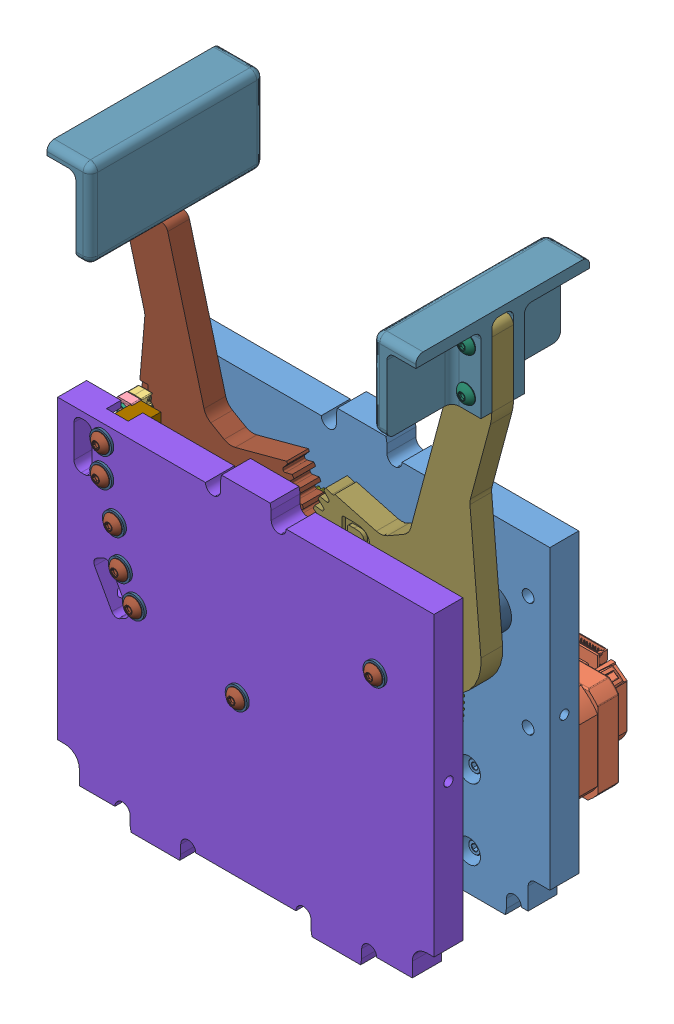
SolidWorks assembly R_ASSY_200_rev3, configuration Default. Lengths in mm.
Overall size (165.1 249.75 130.56).
101 component instances, 30 part files, 189 mates.
Components (placement in the parent):
- R_200_01_rev3-1: R_200_01_rev3 [Default] at (42.4652 115.7578 110.3805) size (165.1 155.57 12.7)
- STP-MTR-17048E-1: STP-MTR-17048E [Default] at (114.3442 119.6359 5.7474) x (-1 0 0) z (0 0 1) size (42.16 62.89 84.58)
- R_200_03_rev2-1: R_200_03_rev2 [Default] at (39.2022 113.0052 142.1305) x (-0.709234 0.704973 0) z (0 0 1) size (6.35 6.35 50.8)
- R_200_04-1: R_200_04 [Default] at (-14.6848 152.2703 142.1305) x (0.39149 -0.920182 0) z (0 0 -1) size (9.53 9.53 50.8)
- R_200_04-2: R_200_04 [Default] at (99.6152 152.2703 142.1305) x (0.332871 0.942972 0) z (0 0 1) size (9.53 9.53 50.8)
- 91116A120_TYPE 18-8 STAINLESS STL OVERSIZED FLAT WASHER-1: 91116A120_TYPE 18-8 STAINLESS STL OVERSIZED FLAT WASHER [91116A120] at (-20.6538 89.9768 116.7305) size (9 9 0.9)
- 91116A120_TYPE 18-8 STAINLESS STL OVERSIZED FLAT WASHER-9: 91116A120_TYPE 18-8 STAINLESS STL OVERSIZED FLAT WASHER [91116A120] at (105.5842 89.9768 116.7305) x (0.949722 0.313094 0) z (0 0 1) size (9 9 0.9)
- 91116A120_TYPE 18-8 STAINLESS STL OVERSIZED FLAT WASHER-11: 91116A120_TYPE 18-8 STAINLESS STL OVERSIZED FLAT WASHER [91116A120] at (105.5842 58.9888 116.7305) x (0.902124 0.431476 0) z (0 0 1) size (9 9 0.9)
- 12t_Steel_Spur_Gear_32_DP_RS775_Motor_217-5859.step-1: 12t_Steel_Spur_Gear_32_DP_RS775_Motor_217-5859.step [Default] at (4.3652 69.7203 125.1283) size (10.98 10.98 19.05)
- 12t_Steel_Spur_Gear_32_DP_RS775_Motor_217-5859.step-2: 12t_Steel_Spur_Gear_32_DP_RS775_Motor_217-5859.step [Default] at (74.0391 69.7203 125.1283) size (10.98 10.98 19.05)
- R_200_05-1: R_200_05 [Default] at (39.2022 113.0052 132.6055) x (-0.958932 0.283637 0) z (0 0 -1) size (103.19 103.19 25.4)
- R_200_02_rev3-1: R_200_02_rev3 [Default] at (42.4652 115.7578 161.1805) size (165.1 155.57 12.7)
- R_200_07_SPCR_rev3-1: R_200_07_SPCR_rev3 [Default] at (39.2022 113.0052 153.243) size (12.7 12.7 7.68)
- R_200_09_SPCR_rev3-3: R_200_09_SPCR_rev3 [Default] at (-14.6848 152.2703 135.7805) x (1 0 0) z (0 0 -1) size (17.46 17.46 12.57)
- R_203_01_rev4-1: R_203_01_rev4 [Default] at (-14.6848 152.2703 142.1305) size (82.51 177.51 9.53)
- R_200_09_SPCR_rev3-4: R_200_09_SPCR_rev3 [Default] at (99.6152 152.2703 123.2075) x (0.999677 -0.025413 0) z (0 0 1) size (17.46 17.46 12.57)
- R_203_02_rev4-1: R_203_02_rev4 [Default] at (99.6152 152.2703 142.1305) x (-1 0 0) z (0 0 -1) size (82.48 176.02 9.53)
- STP-MTR-17048E-2: STP-MTR-17048E [Default] at (44.6703 119.6359 5.7474) x (-1 0 0) z (0 0 1) size (42.16 62.89 84.58)
- 91125A453_18-8 SS FEM THRDED ROUND STANDOFF-1: 91125A453_18-8 SS FEM THRDED ROUND STANDOFF [91125A453] at (-32.103 275.0161 142.1305) x (-1 0 0) z (0 0 1) size (6.35 6.35 10.62)
- 91125A453_18-8 SS FEM THRDED ROUND STANDOFF-2: 91125A453_18-8 SS FEM THRDED ROUND STANDOFF [91125A453] at (-32.103 255.9661 142.1305) x (-0.987351 -0.158553 0) z (0 0 1) size (6.35 6.35 10.62)
- 91125A453_18-8 SS FEM THRDED ROUND STANDOFF-4: 91125A453_18-8 SS FEM THRDED ROUND STANDOFF [91125A453] at (117.0334 275.0161 142.1305) x (-0.34202 0.939693 0) z (0 0 -1) size (6.35 6.35 10.62)
- 91125A453_18-8 SS FEM THRDED ROUND STANDOFF-6: 91125A453_18-8 SS FEM THRDED ROUND STANDOFF [91125A453] at (117.0334 255.9661 142.1305) x (-0.5 0.866025 0) z (0 0 -1) size (6.35 6.35 10.62)
- R_203_05-1: R_203_05 [Default] at (-28.928 268.6661 142.1305) x (0 0 -1) z (1 0 0) size (76.2 38.1 19.05)
- 92949A192_18-8 SS BUTTON HEAD HEX DRIVE SCREW-19: 92949A192_18-8 SS BUTTON HEAD HEX DRIVE SCREW [92949A192] at (-32.103 275.0161 147.9979) x (-0.998312 -0.058087 0) z (0 0 1) size (7.92 7.92 12.15)
- 92949A192_18-8 SS BUTTON HEAD HEX DRIVE SCREW-20: 92949A192_18-8 SS BUTTON HEAD HEX DRIVE SCREW [92949A192] at (-32.103 255.9661 147.9979) x (-0.976474 -0.215637 0) z (0 0 1) size (7.92 7.92 12.15)
- 92949A192_18-8 SS BUTTON HEAD HEX DRIVE SCREW-22: 92949A192_18-8 SS BUTTON HEAD HEX DRIVE SCREW [92949A192] at (-32.103 275.0161 136.2631) x (0.973943 -0.226793 0) z (0 0 -1) size (7.92 7.92 12.15)
- 92949A192_18-8 SS BUTTON HEAD HEX DRIVE SCREW-25: 92949A192_18-8 SS BUTTON HEAD HEX DRIVE SCREW [92949A192] at (-32.103 255.9661 136.2631) x (0.948563 -0.316589 0) z (0 0 -1) size (7.92 7.92 12.15)
- 92949A192_18-8 SS BUTTON HEAD HEX DRIVE SCREW-27: 92949A192_18-8 SS BUTTON HEAD HEX DRIVE SCREW [92949A192] at (117.0334 275.0161 147.9979) x (-0.973943 -0.226793 0) z (0 0 1) size (7.92 7.92 12.15)
- 92949A192_18-8 SS BUTTON HEAD HEX DRIVE SCREW-28: 92949A192_18-8 SS BUTTON HEAD HEX DRIVE SCREW [92949A192] at (117.0334 255.9661 147.9979) x (-0.948563 -0.316589 0) z (0 0 1) size (7.92 7.92 12.15)
- 92949A192_18-8 SS BUTTON HEAD HEX DRIVE SCREW-29: 92949A192_18-8 SS BUTTON HEAD HEX DRIVE SCREW [92949A192] at (117.0334 275.0161 136.2631) x (-0.998312 0.058087 0) z (0 0 -1) size (7.92 7.92 12.15)
- 92949A192_18-8 SS BUTTON HEAD HEX DRIVE SCREW-30: 92949A192_18-8 SS BUTTON HEAD HEX DRIVE SCREW [92949A192] at (117.0334 255.9661 136.2631) x (-0.976474 0.215637 0) z (0 0 -1) size (7.92 7.92 12.15)
- R_203_05-2: R_203_05 [Default] at (113.8584 268.6661 142.1305) x (0 0 1) z (-1 0 0) size (76.2 38.1 19.05)
- 2797T100_LIGHT DUTY DRY-RUNNING THRUST BEARING-1: 2797T100_LIGHT DUTY DRY-RUNNING THRUST BEARING [2797T1] at (39.2022 113.0052 123.8742) x (-0.703019 0.711171 0) z (0 0 1) size (15.88 15.88 1.59)
- 6338K413_OIL-EMBEDDED FLANGED SLEEVE BEARING-1: 6338K413_OIL-EMBEDDED FLANGED SLEEVE BEARING [6338K413] at (39.2022 113.0052 124.668) x (1 0 0) z (0 -1 0) size (12.7 12.7 12.7)
- 6338K413_OIL-EMBEDDED FLANGED SLEEVE BEARING-2: 6338K413_OIL-EMBEDDED FLANGED SLEEVE BEARING [6338K413] at (39.2022 113.0052 153.243) x (0.987351 -0.158553 0) z (0.158553 0.987351 0) size (12.7 12.7 12.7)
- 6338K414_OIL-EMBEDDED FLANGED SLEEVE BEARING-1: 6338K414_OIL-EMBEDDED FLANGED SLEEVE BEARING [6338K414] at (-14.6848 152.2703 135.7805) x (0.998098 0.061654 0) z (0.061654 -0.998098 0) size (17.46 6.35 17.46)
- 6338K414_OIL-EMBEDDED FLANGED SLEEVE BEARING-2: 6338K414_OIL-EMBEDDED FLANGED SLEEVE BEARING [6338K414] at (-14.6848 152.2703 148.4805) x (0.995248 -0.097377 0) z (0.097377 0.995248 0) size (17.46 6.35 17.46)
- 6338K414_OIL-EMBEDDED FLANGED SLEEVE BEARING-4: 6338K414_OIL-EMBEDDED FLANGED SLEEVE BEARING [6338K414] at (99.6152 152.2703 148.4805) x (-0.283434 0.958992 0) z (-0.958992 -0.283434 0) size (17.46 6.35 17.46)
- 6338K414_OIL-EMBEDDED FLANGED SLEEVE BEARING-6: 6338K414_OIL-EMBEDDED FLANGED SLEEVE BEARING [6338K414] at (99.6152 152.2703 135.7805) x (-0.552443 -0.833551 0) z (-0.833551 0.552443 0) size (17.46 6.35 17.46)
- R_200_09_SPCR_rev3-5: R_200_09_SPCR_rev3 [Default] at (99.6152 152.2703 161.0535) x (0.966573 0.25639 0) z (0 0 -1) size (17.46 17.46 12.57)
- R_200_09_SPCR_rev3-7: R_200_09_SPCR_rev3 [Default] at (-14.6848 152.2703 161.0535) x (-0.36579 0.930697 0) z (0 0 -1) size (17.46 17.46 12.57)
- 91116A120_TYPE 18-8 STAINLESS STL OVERSIZED FLAT WASHER-12: 91116A120_TYPE 18-8 STAINLESS STL OVERSIZED FLAT WASHER [91116A120] at (89.5331 85.2143 116.7305) size (9 9 0.9)
- 91292A027_TYPE 18-8 SS SOCKET HEAD CAP SCREW-1: 91292A027_TYPE 18-8 SS SOCKET HEAD CAP SCREW [91292A027] at (89.5331 85.2143 103.6305) x (-0.923728 -0.383049 0) z (0 0 -1) size (5.5 5.5 17.24)
- 91292A027_TYPE 18-8 SS SOCKET HEAD CAP SCREW-8: 91292A027_TYPE 18-8 SS SOCKET HEAD CAP SCREW [91292A027] at (89.5331 54.2263 103.6305) x (-0.923728 -0.383049 0) z (0 0 -1) size (5.5 5.5 17.24)
- 91292A027_TYPE 18-8 SS SOCKET HEAD CAP SCREW-9: 91292A027_TYPE 18-8 SS SOCKET HEAD CAP SCREW [91292A027] at (-11.1288 85.2143 103.6305) x (-0.923728 -0.383049 0) z (0 0 -1) size (5.5 5.5 17.24)
- 91292A027_TYPE 18-8 SS SOCKET HEAD CAP SCREW-10: 91292A027_TYPE 18-8 SS SOCKET HEAD CAP SCREW [91292A027] at (58.5451 85.2143 103.6305) x (-0.923728 -0.383049 0) z (0 0 -1) size (5.5 5.5 17.24)
- 91292A027_TYPE 18-8 SS SOCKET HEAD CAP SCREW-11: 91292A027_TYPE 18-8 SS SOCKET HEAD CAP SCREW [91292A027] at (58.5451 54.2263 103.6305) x (-0.923728 -0.383049 0) z (0 0 -1) size (5.5 5.5 17.24)
- 91292A027_TYPE 18-8 SS SOCKET HEAD CAP SCREW-12: 91292A027_TYPE 18-8 SS SOCKET HEAD CAP SCREW [91292A027] at (-11.1288 54.2263 103.6305) x (-0.923728 -0.383049 0) z (0 0 -1) size (5.5 5.5 17.24)
- 91292A027_TYPE 18-8 SS SOCKET HEAD CAP SCREW-13: 91292A027_TYPE 18-8 SS SOCKET HEAD CAP SCREW [91292A027] at (19.8592 54.2263 103.6305) x (-0.923728 -0.383049 0) z (0 0 -1) size (5.5 5.5 17.24)
- 91292A027_TYPE 18-8 SS SOCKET HEAD CAP SCREW-14: 91292A027_TYPE 18-8 SS SOCKET HEAD CAP SCREW [91292A027] at (19.8592 85.2143 103.6305) x (-0.923728 -0.383049 0) z (0 0 -1) size (5.5 5.5 17.24)
- 91116A120_TYPE 18-8 STAINLESS STL OVERSIZED FLAT WASHER-19: 91116A120_TYPE 18-8 STAINLESS STL OVERSIZED FLAT WASHER [91116A120] at (89.5331 54.2263 116.7305) size (9 9 0.9)
- 91116A120_TYPE 18-8 STAINLESS STL OVERSIZED FLAT WASHER-20: 91116A120_TYPE 18-8 STAINLESS STL OVERSIZED FLAT WASHER [91116A120] at (-11.1288 85.2143 116.7305) size (9 9 0.9)
- 91116A120_TYPE 18-8 STAINLESS STL OVERSIZED FLAT WASHER-21: 91116A120_TYPE 18-8 STAINLESS STL OVERSIZED FLAT WASHER [91116A120] at (58.5451 85.2143 116.7305) size (9 9 0.9)
- 91116A120_TYPE 18-8 STAINLESS STL OVERSIZED FLAT WASHER-22: 91116A120_TYPE 18-8 STAINLESS STL OVERSIZED FLAT WASHER [91116A120] at (58.5451 54.2263 116.7305) size (9 9 0.9)
- 91116A120_TYPE 18-8 STAINLESS STL OVERSIZED FLAT WASHER-23: 91116A120_TYPE 18-8 STAINLESS STL OVERSIZED FLAT WASHER [91116A120] at (-11.1288 54.2263 116.7305) size (9 9 0.9)
- 91116A120_TYPE 18-8 STAINLESS STL OVERSIZED FLAT WASHER-24: 91116A120_TYPE 18-8 STAINLESS STL OVERSIZED FLAT WASHER [91116A120] at (19.8592 54.2263 116.7305) size (9 9 0.9)
- 91116A120_TYPE 18-8 STAINLESS STL OVERSIZED FLAT WASHER-25: 91116A120_TYPE 18-8 STAINLESS STL OVERSIZED FLAT WASHER [91116A120] at (19.8592 85.2143 116.7305) size (9 9 0.9)
- dc1c-a1aa-1: dc1c-a1aa [Default] at (-27.4348 169.2553 154.8305) x (0 1 0) z (-1 0 0) size (19.85 14.96 6.45)
  - dc1c-a1aa_01-1: dc1c-a1aa_01 [Default] at origin size (5.58 3.61 5.58)
  - dc1c-a1aa_02-1: dc1c-a1aa_02 [Default] at origin size (19.73 5.96 6.26)
  - dc1c-a1aa_03-1: dc1c-a1aa_03 [Default] at origin size (19.85 3.9 6.45)
  - dc1c-a1aa_04-1: dc1c-a1aa_04 [Default] at origin size (1.69 3.85 2.68)
  - dc1c-a1aa_05-1: dc1c-a1aa_05 [Default] at origin size (1.69 3.85 2.68)
  - dc1c-a1aa_06-1: dc1c-a1aa_06 [Default] at origin size (1.69 3.85 2.68)
- 92095A104_BUTTON HEAD HEX DRIVE SCREW-1: 92095A104_BUTTON HEAD HEX DRIVE SCREW [92095A104] at (-31.5598 169.2553 154.8305) x (0 0 1) z (-1 0 0) size (3.8 3.8 11.02)
- R_200_10-2: R_200_10 [Default] at (-20.241 174.0203 167.5305) x (0 0 1) z (-1 0 0) size (14.29 19.05 9.53)
- 92095A104_BUTTON HEAD HEX DRIVE SCREW-2: 92095A104_BUTTON HEAD HEX DRIVE SCREW [92095A104] at (-31.5598 178.7853 154.8305) x (0 -0.984808 -0.173648) z (-1 0 0) size (3.8 3.8 11.02)
- R_200_10-3: R_200_10 [Default] at (-8.9998 130.5536 167.5305) x (0 0 1) z (-0.87462 -0.48481 0) size (14.29 19.05 9.53)
- dc1c-a1aa-2: dc1c-a1aa [Default] at (-17.6017 131.2336 154.8305) x (0.48481 -0.87462 0) z (0.87462 0.48481 0) size (19.85 14.96 6.45)
  - dc1c-a1aa_01-1: dc1c-a1aa_01 [Default] at origin size (5.58 3.61 5.58)
  - dc1c-a1aa_02-1: dc1c-a1aa_02 [Default] at origin size (19.73 5.96 6.26)
  - dc1c-a1aa_03-1: dc1c-a1aa_03 [Default] at origin size (19.85 3.9 6.45)
  - dc1c-a1aa_04-1: dc1c-a1aa_04 [Default] at origin size (1.69 3.85 2.68)
  - dc1c-a1aa_05-1: dc1c-a1aa_05 [Default] at origin size (1.69 3.85 2.68)
  - dc1c-a1aa_06-1: dc1c-a1aa_06 [Default] at origin size (1.69 3.85 2.68)
- 92095A104_BUTTON HEAD HEX DRIVE SCREW-3: 92095A104_BUTTON HEAD HEX DRIVE SCREW [92095A104] at (-21.2095 129.2337 154.8305) x (-0.34402 0.620628 0.704607) z (-0.87462 -0.48481 0) size (3.8 3.8 11.02)
- 92095A104_BUTTON HEAD HEX DRIVE SCREW-5: 92095A104_BUTTON HEAD HEX DRIVE SCREW [92095A104] at (-16.5893 120.8986 154.8305) x (-0.449843 0.811539 -0.372887) z (-0.87462 -0.48481 0) size (3.8 3.8 11.02)
- 92141A009_TYPE 18-8 STAINLESS STEEL FLAT WASHER-5: 92141A009_TYPE 18-8 STAINLESS STEEL FLAT WASHER [92141A009] at (-20.241 180.3703 174.8965) x (-0.777574 -0.628792 0) z (0.628792 -0.777574 0) size (9.53 1.02 9.53)
- 92949A194_18-8 SS BUTTON HEAD HEX DRIVE SCREW-12: 92949A194_18-8 SS BUTTON HEAD HEX DRIVE SCREW [92949A194] at (-20.241 180.3703 169.6514) x (0.994367 -0.105992 0) z (0 0 1) size (7.92 7.92 15.34)
- 92141A009_TYPE 18-8 STAINLESS STEEL FLAT WASHER-6: 92141A009_TYPE 18-8 STAINLESS STEEL FLAT WASHER [92141A009] at (-20.241 167.6703 174.8965) x (-0.668041 -0.744124 0) z (0.744124 -0.668041 0) size (9.53 1.02 9.53)
- 92949A194_18-8 SS BUTTON HEAD HEX DRIVE SCREW-17: 92949A194_18-8 SS BUTTON HEAD HEX DRIVE SCREW [92949A194] at (-20.241 167.6703 169.6514) x (0.964983 -0.262311 0) z (0 0 1) size (7.92 7.92 15.34)
- 92141A009_TYPE 18-8 STAINLESS STEEL FLAT WASHER-7: 92141A009_TYPE 18-8 STAINLESS STEEL FLAT WASHER [92141A009] at (-14.6848 152.2703 174.8965) x (-0.567853 -0.82313 0) z (0.82313 -0.567853 0) size (9.53 1.02 9.53)
- 92949A194_18-8 SS BUTTON HEAD HEX DRIVE SCREW-18: 92949A194_18-8 SS BUTTON HEAD HEX DRIVE SCREW [92949A194] at (-14.6848 152.2703 169.6514) x (0.923728 -0.383049 0) z (0 0 1) size (7.92 7.92 15.34)
- 92141A009_TYPE 18-8 STAINLESS STEEL FLAT WASHER-8: 92141A009_TYPE 18-8 STAINLESS STEEL FLAT WASHER [92141A009] at (-12.0783 136.1074 174.8965) x (-0.488654 -0.872477 0) z (0.872477 -0.488654 0) size (9.53 1.02 9.53)
- 92949A194_18-8 SS BUTTON HEAD HEX DRIVE SCREW-19: 92949A194_18-8 SS BUTTON HEAD HEX DRIVE SCREW [92949A194] at (-12.0783 136.1074 169.6514) x (0.884001 -0.467484 0) z (0 0 1) size (7.92 7.92 15.34)
- 92141A009_TYPE 18-8 STAINLESS STEEL FLAT WASHER-9: 92141A009_TYPE 18-8 STAINLESS STEEL FLAT WASHER [92141A009] at (-5.9212 124.9998 174.8965) x (-0.440433 -0.897785 0) z (0.897785 -0.440433 0) size (9.53 1.02 9.53)
- 92949A194_18-8 SS BUTTON HEAD HEX DRIVE SCREW-20: 92949A194_18-8 SS BUTTON HEAD HEX DRIVE SCREW [92949A194] at (-5.9212 124.9998 169.6514) x (0.857241 -0.514915 0) z (0 0 1) size (7.92 7.92 15.34)
- 92141A009_TYPE 18-8 STAINLESS STEEL FLAT WASHER-10: 92141A009_TYPE 18-8 STAINLESS STEEL FLAT WASHER [92141A009] at (39.2022 113.0052 174.8965) x (-0.431679 -0.902027 0) z (0.902027 -0.431679 0) size (9.53 1.02 9.53)
- 92949A194_18-8 SS BUTTON HEAD HEX DRIVE SCREW-16: 92949A194_18-8 SS BUTTON HEAD HEX DRIVE SCREW [92949A194] at (39.2022 113.0052 169.6514) x (0.852192 -0.523229 0) z (0 0 1) size (7.92 7.92 15.34)
- 92141A009_TYPE 18-8 STAINLESS STEEL FLAT WASHER-11: 92141A009_TYPE 18-8 STAINLESS STEEL FLAT WASHER [92141A009] at (99.6152 152.2703 174.8965) x (-0.468067 -0.883693 0) z (0.883693 -0.468067 0) size (9.53 1.02 9.53)
- 92949A194_18-8 SS BUTTON HEAD HEX DRIVE SCREW-11: 92949A194_18-8 SS BUTTON HEAD HEX DRIVE SCREW [92949A194] at (99.6152 152.2703 169.6514) x (0.872799 -0.488079 0) z (0 0 1) size (7.92 7.92 15.34)
- 92141A009_TYPE 18-8 STAINLESS STEEL FLAT WASHER-14: 92141A009_TYPE 18-8 STAINLESS STEEL FLAT WASHER [92141A009] at (-14.6848 152.2703 109.3645) x (-0.484215 -0.874949 0) z (-0.874949 0.484215 0) size (9.53 1.02 9.53)
- 92949A194_18-8 SS BUTTON HEAD HEX DRIVE SCREW-22: 92949A194_18-8 SS BUTTON HEAD HEX DRIVE SCREW [92949A194] at (-14.6848 152.2703 114.6096) x (-0.277052 0.960855 0) z (0 0 -1) size (7.92 7.92 15.34)
- 92141A009_TYPE 18-8 STAINLESS STEEL FLAT WASHER-16: 92141A009_TYPE 18-8 STAINLESS STEEL FLAT WASHER [92141A009] at (39.2022 113.0052 109.3645) x (-0.324925 -0.94574 0) z (-0.94574 0.324925 0) size (9.53 1.02 9.53)
- 92949A194_18-8 SS BUTTON HEAD HEX DRIVE SCREW-24: 92949A194_18-8 SS BUTTON HEAD HEX DRIVE SCREW [92949A194] at (39.2022 113.0052 114.6096) x (-0.439693 0.898148 0) z (0 0 -1) size (7.92 7.92 15.34)
- 92141A009_TYPE 18-8 STAINLESS STEEL FLAT WASHER-18: 92141A009_TYPE 18-8 STAINLESS STEEL FLAT WASHER [92141A009] at (99.6152 152.2703 109.3645) x (-0.155763 -0.987795 0) z (-0.987795 0.155763 0) size (9.53 1.02 9.53)
- 92949A194_18-8 SS BUTTON HEAD HEX DRIVE SCREW-26: 92949A194_18-8 SS BUTTON HEAD HEX DRIVE SCREW [92949A194] at (99.6152 152.2703 114.6096) x (-0.588975 0.808151 0) z (0 0 -1) size (7.92 7.92 15.34)
- 93365A142_HEAT-SET INSERTS FOR PLASTICS-1: 93365A142_HEAT-SET INSERTS FOR PLASTICS [93365A142] at (115.4902 114.0178 110.3805) x (-0.923728 -0.383049 0) z (0.383049 -0.923728 0) size (6.35 8.46 6.35)
- 93365A142_HEAT-SET INSERTS FOR PLASTICS-2: 93365A142_HEAT-SET INSERTS FOR PLASTICS [93365A142] at (-30.5598 114.0178 110.3805) x (-0.923728 -0.383049 0) z (0.383049 -0.923728 0) size (6.35 8.46 6.35)
- 93365A142_HEAT-SET INSERTS FOR PLASTICS-3: 93365A142_HEAT-SET INSERTS FOR PLASTICS [93365A142] at (-30.5598 164.0178 110.3805) x (-0.923728 -0.383049 0) z (0.383049 -0.923728 0) size (6.35 8.46 6.35)
- 93365A142_HEAT-SET INSERTS FOR PLASTICS-4: 93365A142_HEAT-SET INSERTS FOR PLASTICS [93365A142] at (115.4902 164.0178 110.3805) x (-0.923728 -0.383049 0) z (0.383049 -0.923728 0) size (6.35 8.46 6.35)
Mates (geometry in assembly coordinates):
- Concentric1: concentric: cylinder of R_200_01_rev3-1 through (-5.1598 74.4828 78.9496) axis (0 0 1) radius 11.1125; cylinder of ? through (-5.1598 74.4828 110.3805) axis (0 0 1) radius 10.9982
- Coincident1: coincident: plane of R_200_01_rev3-1 through (42.4652 115.7578 110.3805) normal (0 0 -1); plane of ? through (-5.1598 74.4828 110.3805) normal (0 0 1)
- Concentric2: concentric: cylinder of R_200_01_rev3-1 through (10.3342 89.9768 123.0805) axis (0 0 1) radius 1.7; cylinder of ? through (10.3342 89.9768 112.9205) axis (0 0 -1) radius 1.0922
- Concentric3: concentric: cylinder of R_200_01_rev3-1 through (-20.6538 89.9768 123.0805) axis (0 0 1) radius 1.7; cylinder of ? through (-20.6538 89.9768 112.9205) axis (0 0 -1) radius 1.0922
- Concentric4: concentric: cylinder of R_200_01_rev3-1 through (-20.6538 58.9888 123.0805) axis (0 0 1) radius 1.7; cylinder of ? through (-20.6538 58.9888 112.9205) axis (0 0 -1) radius 1.0922
- Concentric5: concentric: cylinder of R_200_01_rev3-1 through (10.3342 58.9888 123.0805) axis (0 0 1) radius 1.7; cylinder of ? through (10.3342 58.9888 112.9205) axis (0 0 -1) radius 1.0922
- Coincident7: coincident: plane of 91116A120_TYPE 18-8 STAINLESS STL OVERSIZED FLAT WASHER-1 through (-20.6538 89.9768 117.6305) normal (0 0 1); plane of 91292A027_TYPE 18-8 SS SOCKET HEAD CAP SCREW-1 through (89.5331 85.2143 117.6305) normal (0 0 -1)
- Coincident16: coincident: plane of 91116A120_TYPE 18-8 STAINLESS STL OVERSIZED FLAT WASHER-11 through (105.5842 58.9888 117.6305) normal (0 0 1); plane of 91292A027_TYPE 18-8 SS SOCKET HEAD CAP SCREW-9 through (-11.1288 85.2143 117.6305) normal (0 0 -1)
- Concentric32: concentric: cylinder of ? through (-5.1598 74.4828 110.3805) axis (0 0 1) radius 2.4994; cylinder of 12t_Steel_Spur_Gear_32_DP_RS775_Motor_217-5859.step-1 through (-5.1598 74.4828 115.2065) axis (0 0 1) radius 2.48
- Coincident28: coincident: plane of ? through (-5.1598 74.4828 134.2565) normal (0 0 1); plane of 12t_Steel_Spur_Gear_32_DP_RS775_Motor_217-5859.step-1 through (-5.1598 74.4828 134.2565) normal (0 0 1)
- Concentric33: concentric: cylinder of STP-MTR-17048E-1 through (74.0391 69.7203 110.3805) axis (0 0 1) radius 2.4994; cylinder of 12t_Steel_Spur_Gear_32_DP_RS775_Motor_217-5859.step-2 through (74.0391 69.7203 115.2065) axis (0 0 1) radius 2.48
- Coincident29: coincident: plane of STP-MTR-17048E-1 through (74.0391 69.7203 134.2565) normal (0 0 1); plane of 12t_Steel_Spur_Gear_32_DP_RS775_Motor_217-5859.step-2 through (74.0391 69.7203 134.2565) normal (0 0 1)
- Concentric39: concentric: cylinder of R_200_04-1 through (-8.3348 146.2865 167.5305) axis (0 0 -1) radius 4.7625; cylinder of ? through (-8.3348 146.2865 150.068) axis (0 0 -1) radius 4.7752
- Concentric40: concentric: cylinder of R_200_04-2 through (105.9652 146.2865 167.5305) axis (0 0 -1) radius 4.7625; cylinder of ? through (105.9652 146.2865 137.368) axis (0 0 1) radius 4.7752
- Coincident42: coincident: plane of R_200_01_rev3-1 through (42.4652 115.7578 110.3805) normal (0 0 -1); plane of ? through (90.2172 26.8578 110.3805) normal (0 0 1)
- Coincident46: coincident: plane of R_200_01_rev3-1 through (42.4652 115.7578 110.3805) normal (0 0 -1); plane of ? through (37.8297 198.3078 110.3805) normal (0 0 1)
- Coincident47: coincident: plane of R_200_01_rev3-1 through (-40.0848 191.9578 123.0805) normal (0 1 0); plane of ? through (130.0952 191.9578 53.3575) normal (0 -1 0)
- Coincident49: coincident: plane of R_200_01_rev3-1 through (-40.0848 39.5578 123.0805) normal (-1 0 0); plane of ? through (-40.0848 191.9578 250.2075) normal (-1 0 0)
- Coincident50: coincident: plane of R_200_01_rev3-1 through (125.0152 39.5578 123.0805) normal (1 0 0); plane of ? through (125.0152 191.9578 250.2075) normal (1 0 0)
- Coincident51: coincident: plane of R_200_01_rev3-1 through (-40.0848 39.5578 123.0805) normal (-1 0 0); plane of ? through (-40.0848 26.8578 250.2075) normal (-1 0 0)
- Coincident52: coincident: plane of ? through (-45.1648 33.2078 250.2075) normal (0 -1 0); plane of ? through (-45.1648 33.2078 253.3825) normal (0 1 0)
- Coincident53: coincident: plane of ? through (-45.1648 26.8578 53.3575) normal (-1 0 0); plane of ? through (-45.1648 204.9118 151.7825) normal (1 0 0)
- Coincident55: coincident: plane of ? through (130.0952 33.2078 250.2075) normal (0 -1 0); plane of ? through (130.0952 33.2078 50.1825) normal (0 1 0)
- Coincident56: coincident: plane of ? through (130.0952 26.8578 53.3575) normal (1 0 0); plane of ? through (130.0952 204.9118 151.7825) normal (-1 0 0)
- Coincident58: coincident: plane of ? through (-39.8308 14.4118 262.9075) normal (0 0 1); plane of ? through (124.7612 14.4118 262.9075) normal (0 0 1)
- Width1: width: plane of ? through (42.4652 33.2078 250.2075) normal (0 0 1); plane of ? through (42.4652 33.2078 53.3575) normal (0 0 -1); plane of ? through (124.7612 14.4118 262.9075) normal (0 0 1); plane of ? through (124.7612 14.4118 40.6575) normal (0 0 -1)
- Width2: width: plane of R_200_01_rev3-1 through (42.4652 115.7578 123.0805) normal (0 0 1); plane of R_200_01_rev3-1 through (42.4652 115.7578 110.3805) normal (0 0 -1); plane of ? through (-14.5578 26.8578 123.3345) normal (0 0 -1); plane of ? through (-14.5578 26.8578 110.3805) normal (0 0 1)
- Coincident61: coincident: plane of 6338K413_OIL-EMBEDDED FLANGED SLEEVE BEARING-2 through (39.2022 113.0052 153.243) normal (0 0 1); plane of R_200_07_SPCR_rev3-1 through (39.2022 113.0052 153.243) normal (0 0 -1)
- Concentric48: concentric: cylinder of R_200_03_rev2-1 through (39.2022 113.0052 167.5305) axis (0 0 -1) radius 3.175; cylinder of R_200_07_SPCR_rev3-1 through (39.2022 113.0052 160.9265) axis (0 0 -1) radius 3.302
- Coincident63: coincident: plane of ? through (-32.0288 226.3803 150.068) normal (0 0 1); plane of ? through (-8.3348 146.2865 150.068) normal (0 0 -1)
- Concentric49: concentric: cylinder of R_200_04-1 through (-8.3348 146.2865 167.5305) axis (0 0 -1) radius 4.7625; cylinder of ? through (-8.3348 146.2865 161.1805) axis (0 0 -1) radius 4.8895
- Coincident66: coincident: plane of R_200_01_rev3-1 through (42.4652 115.7578 123.0805) normal (0 0 1); plane of ? through (-8.3348 146.2865 123.0805) normal (0 0 -1)
- Concentric51: concentric: cylinder of R_200_04-1 through (-8.3348 146.2865 167.5305) axis (0 0 -1) radius 4.7625; cylinder of ? through (-8.3348 146.2865 137.114) axis (0 0 -1) radius 4.8895
- Concentric53: concentric: cylinder of R_200_01_rev3-1 through (18.4368 98.0794 123.0805) axis (0 0 1) radius 1.7; cylinder of ? through (18.4368 98.0794 110.3805) axis (0 0 -1) radius 2.54
- Concentric56: concentric: cylinder of R_200_01_rev3-1 through (18.4368 50.8862 123.0805) axis (0 0 1) radius 1.7; cylinder of ? through (18.4368 50.8862 110.3805) axis (0 0 -1) radius 2.54
- Concentric57: concentric: cylinder of R_200_01_rev3-1 through (-28.7564 98.0794 123.0805) axis (0 0 1) radius 1.7; cylinder of ? through (-28.7564 98.0794 110.3805) axis (0 0 -1) radius 2.54
- Concentric58: concentric: cylinder of R_200_01_rev3-1 through (-28.7564 50.8862 123.0805) axis (0 0 1) radius 1.7; cylinder of ? through (-28.7564 50.8862 110.3805) axis (0 0 -1) radius 2.54
- Coincident68: coincident: plane of R_200_01_rev3-1 through (42.4652 115.7578 110.3805) normal (0 0 -1); plane of ? through (-5.1598 74.4828 110.3805) normal (0 0 1)
- Concentric60: concentric: cylinder of R_200_04-1 through (-14.6848 152.2703 116.7305) axis (0 0 1) radius 4.7625; cylinder of R_200_09_SPCR_rev3-3 through (-14.6848 152.2703 123.2075) axis (0 0 1) radius 4.8895
- Coincident71: coincident: plane of 6338K414_OIL-EMBEDDED FLANGED SLEEVE BEARING-1 through (-14.6848 152.2703 135.7805) normal (0 0 -1); plane of R_200_09_SPCR_rev3-3 through (-14.6848 152.2703 135.7805) normal (0 0 1)
- Concentric64: concentric: cylinder of R_200_04-2 through (99.6152 152.2703 167.5305) axis (0 0 -1) radius 4.7625; cylinder of R_200_09_SPCR_rev3-4 through (99.6152 152.2703 135.7805) axis (0 0 -1) radius 4.8895
- Coincident75: coincident: plane of R_200_09_SPCR_rev3-4 through (99.6152 152.2703 135.7805) normal (0 0 1); plane of 6338K414_OIL-EMBEDDED FLANGED SLEEVE BEARING-6 through (99.6152 152.2703 135.7805) normal (0 0 -1)
- LimitAngle1: limit planar angle: plane of R_203_01_rev4-1 through (10.7152 150.6701 145.3055) normal (0 1 0); plane of R_200_01_rev3-1 through (-40.0848 187.1953 123.0805) normal (0 1 0)
- Angle2: planar angle: plane of R_200_01_rev3-1 through (-40.0848 187.1953 123.0805) normal (0 1 0); plane of R_203_02_rev4-1 through (74.2152 150.6701 145.3055) normal (0 1 0)
- Concentric67: concentric: cylinder of R_200_01_rev3-1 through (99.6152 152.2703 116.7305) axis (0 0 1) radius 4.7752; cylinder of R_200_04-2 through (99.6152 152.2703 167.5305) axis (0 0 -1) radius 4.7625
- Concentric68: concentric: cylinder of R_200_01_rev3-1 through (-14.6848 152.2703 116.7305) axis (0 0 1) radius 4.7752; cylinder of R_200_04-1 through (-14.6848 152.2703 116.7305) axis (0 0 1) radius 4.7625
- Coincident77: coincident: plane of R_200_01_rev3-1 through (-14.6848 152.2703 116.7305) normal (0 0 1); plane of R_200_04-1 through (-14.6848 152.2703 116.7305) normal (0 0 -1)
- Coincident80: coincident: plane of R_200_01_rev3-1 through (99.6152 152.2703 116.7305) normal (0 0 1); plane of R_200_04-2 through (99.6152 152.2703 116.7305) normal (0 0 -1)
- Coincident81: coincident: plane of R_200_01_rev3-1 through (39.2022 113.0052 116.7305) normal (0 0 1); plane of R_200_03_rev2-1 through (39.2022 113.0052 116.7305) normal (0 0 -1)
- Concentric69: concentric: cylinder of R_200_01_rev3-1 through (39.2022 113.0052 116.7305) axis (0 0 1) radius 3.1877; cylinder of R_200_03_rev2-1 through (39.2022 113.0052 167.5305) axis (0 0 -1) radius 3.175
- Concentric70: concentric: cylinder of STP-MTR-17048E-1 through (58.5451 54.2263 110.3805) axis (0 0 -1) radius 1.0922; cylinder of R_200_01_rev3-1 through (58.5451 54.2263 123.0805) axis (0 0 1) radius 1.7
- Coincident82: coincident: plane of R_200_01_rev3-1 through (42.4652 115.7578 110.3805) normal (0 0 -1); plane of STP-MTR-17048E-1 through (74.0391 69.7203 110.3805) normal (0 0 1)
- Concentric74: concentric: cylinder of STP-MTR-17048E-2 through (-11.1288 54.2263 110.3805) axis (0 0 -1) radius 1.0922; cylinder of R_200_01_rev3-1 through (-11.1288 54.2263 123.0805) axis (0 0 1) radius 1.7
- Concentric78: concentric: cylinder of 12t_Steel_Spur_Gear_32_DP_RS775_Motor_217-5859.step-1 through (4.3652 69.7203 115.2065) axis (0 0 1) radius 2.48; cylinder of STP-MTR-17048E-2 through (4.3652 69.7203 110.3805) axis (0 0 1) radius 2.4994
- Coincident84: coincident: plane of 12t_Steel_Spur_Gear_32_DP_RS775_Motor_217-5859.step-1 through (4.3652 69.7203 134.2565) normal (0 0 1); plane of STP-MTR-17048E-2 through (4.3652 69.7203 134.2565) normal (0 0 1)
- Coincident85: coincident: plane of R_200_01_rev3-1 through (42.4652 115.7578 110.3805) normal (0 0 -1); plane of STP-MTR-17048E-2 through (4.3652 69.7203 110.3805) normal (0 0 1)
- Concentric79: concentric: cylinder of R_200_04-1 through (-14.6848 152.2703 116.7305) axis (0 0 1) radius 4.7625; cylinder of R_200_02_rev3-1 through (-14.6848 152.2703 167.5305) axis (0 0 -1) radius 4.7625
- Concentric80: concentric: cylinder of R_200_04-2 through (99.6152 152.2703 167.5305) axis (0 0 -1) radius 4.7625; cylinder of R_200_02_rev3-1 through (99.6152 152.2703 167.5305) axis (0 0 -1) radius 4.7625
- Concentric81: concentric: cylinder of R_200_03_rev2-1 through (39.2022 113.0052 167.5305) axis (0 0 -1) radius 3.175; cylinder of R_200_02_rev3-1 through (39.2022 113.0052 167.5305) axis (0 0 -1) radius 3.175
- Coincident87: coincident: plane of R_200_04-1 through (-14.6848 152.2703 167.5305) normal (0 0 1); plane of R_200_02_rev3-1 through (-14.6848 152.2703 167.5305) normal (0 0 -1)
- Coincident103: coincident: plane of R_200_01_rev3-1 through (-40.0848 44.3203 123.0805) normal (0 -1 0); plane of R_200_02_rev3-1 through (-40.0848 44.3203 173.8805) normal (0 -1 0)
- Concentric108: concentric: cylinder of R_203_01_rev4-1 through (-32.103 275.0161 146.893) axis (0 0 1) radius 3.175; cylinder of 91125A453_18-8 SS FEM THRDED ROUND STANDOFF-1 through (-32.103 275.0161 146.893) axis (0 0 -1) radius 3.175
- Width3: width: plane of 91125A453_18-8 SS FEM THRDED ROUND STANDOFF-1 through (-32.103 275.0161 146.893) normal (0 0 1); plane of 91125A453_18-8 SS FEM THRDED ROUND STANDOFF-1 through (-32.103 275.0161 137.368) normal (0 0 -1); plane of R_203_01_rev4-1 through (-14.6848 152.2703 137.368) normal (0 0 -1); plane of R_203_01_rev4-1 through (-14.6848 152.2703 146.893) normal (0 0 1)
